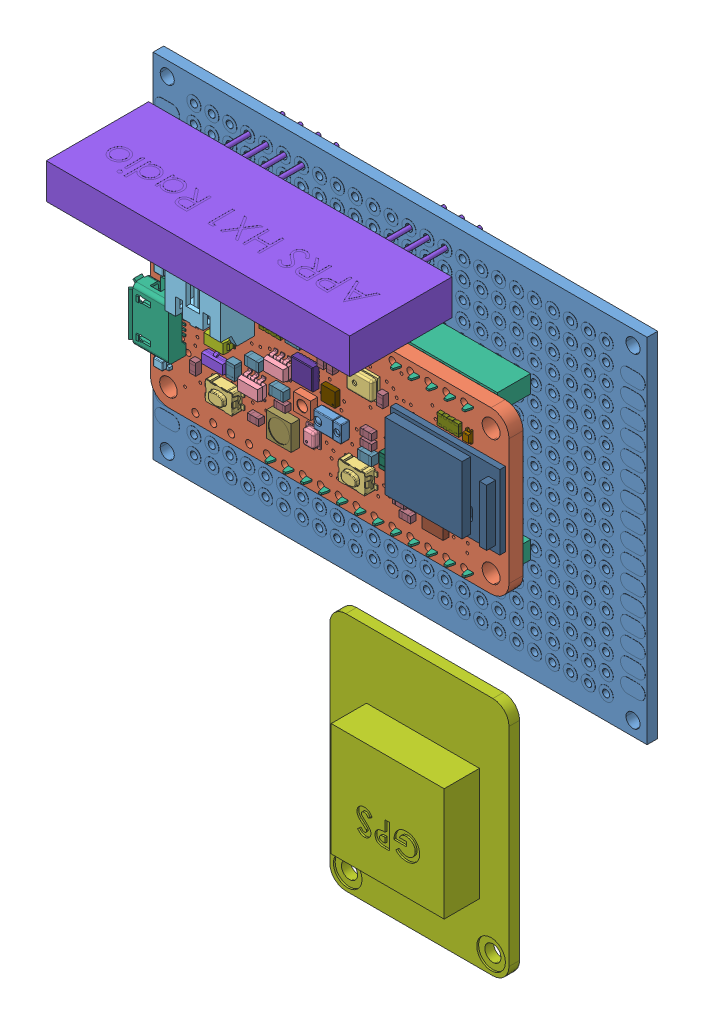
SolidWorks assembly protoboard_assembly, configuration Default. Lengths in mm.
Overall size (70 82.89 26.5).
48 component instances, 26 part files, 16 mates.
Components (placement in the parent):
- protoboard-1: protoboard [Default] at (39.9767 30.2093 49.9679) size (70 50 1.55)
- feather_sense-1: feather_sense [Default] at (11.5967 19.6493 56.4679) size (51.35 22.86 6.79)
  - feather_sense.step-1: feather_sense.step [Default] at origin size (51.35 22.86 6.79)
    - PCB Component.step-1: PCB Component.step [Default] at origin size (51.35 22.86 6.79)
      - Board.step-1: Board.step [Default] at origin size (50.8 22.86 1.99)
      - KMR2.step-1: KMR2.step [Default] at (11.1 6.223 1.99) size (4.6 2.8 1.94)
      - KMR2.step-2: KMR2.step [Default] at (29.934 5.855 1.99) size (4.6 2.8 1.94)
      - AP2112(3.3V).step-1: AP2112(3.3V).step [Default] at (15.138 9.144 1.99) x (-1 0 0) z (0 0 1) size (3 3 1.4)
      - AP2112(3.3V).step-2: AP2112(3.3V).step [Default] at (18.783 13.386 1.99) x (-1 0 0) z (0 0 1) size (3 3 1.4)
      - RED.step-1: RED.step [Default] at (2.083 5.639 1.99) x (0 -1 0) z (0 0 1) size (1.25 2.02 1.1)
      - RED.step-2: RED.step [Default] at (2.222 17.272 1.99) x (0 1 0) z (0 0 1) size (1.25 2.02 1.1)
      - 4u20329.step-1: 4u20329.step [Default] at (4.445 11.43 1.99) x (0 -1 0) z (0 0 1) size (8.8 5.6 3)
      - MBR054.step-1: MBR054.step [Default] at (10.262 12.395 1.99) x (-1 0 0) z (0 0 1) size (3.6 1.4 1.35)
      - DMG2305.step-1: DMG2305.step [Default] at (9.817 9.55 1.99) size (3.04 2.64 1.12)
      - BLUE.step-1: BLUE.step [Default] at (45.339 18.034 1.99) x (-1 0 0) z (0 0 1) size (0.79 1.6 0.71)
      - MDBT50.step-1: MDBT50.step [Default] at (42.545 11.43 1.99) x (0 -1 0) z (0 0 1) size (10.5 15.5 2.05)
      - GD25Q16.step-1: GD25Q16.step [Default] at (40.767 4.953 1.99) x (-1 0 0) z (0 0 1) size (3 2 0.8)
      - WS2812B3535.step-1: WS2812B3535.step [Default] at (19.387 6.145 1.99) x (-1 0 0) z (0 0 1) size (3.5 3.5 1.2)
      - 2.2K.step-1: 2.2K.step [Default] at (19.075 8.788 1.99) size (1.6 0.9 0.8)
      - 2.2K.step-2: 2.2K.step [Default] at (31.306 10.198 1.99) size (1.6 0.9 0.8)
      - 2.2K.step-3: 2.2K.step [Default] at (6.756 7.379 1.99) x (0 1 0) z (0 0 1) size (1.6 0.9 0.8)
      - 2.2K.step-4: 2.2K.step [Default] at (15.316 5.309 1.99) size (1.6 0.9 0.8)
      - 2.2K.step-5: 2.2K.step [Default] at (35.878 5.398 1.99) size (1.6 0.9 0.8)
      - 2.2K.step-6: 2.2K.step [Default] at (36.83 4.128 1.99) size (1.6 0.9 0.8)
      - 2.2K.step-7: 2.2K.step [Default] at (33.274 16.637 1.99) x (0 1 0) z (0 0 1) size (1.6 0.9 0.8)
      - 2.2K.step-8: 2.2K.step [Default] at (26.162 17.208 1.99) x (0 -1 0) z (0 0 1) size (1.6 0.9 0.8)
      - 2.2K.step-9: 2.2K.step [Default] at (31.306 11.494 1.99) size (1.6 0.9 0.8)
      - 2.2K.step-10: 2.2K.step [Default] at (24.828 17.208 1.99) x (0 -1 0) z (0 0 1) size (1.6 0.9 0.8)
      - 2.2K.step-11: 2.2K.step [Default] at (5.715 19.685 1.99) x (0 -1 0) z (0 0 1) size (1.6 0.9 0.8)
      - 10uF.step-1: 10uF.step [Default] at (18.796 10.376 1.99) size (2 1.25 1)
      - 10uF.step-2: 10uF.step [Default] at (21.082 17.907 1.99) x (-1 0 0) z (0 0 1) size (2 1.25 1)
      - 10uF.step-3: 10uF.step [Default] at (12.294 9.855 1.99) x (0 1 0) z (0 0 1) size (2 1.25 1)
      - 10uF.step-4: 10uF.step [Default] at (31.306 8.712 1.99) size (2 1.25 1)
      - 10uF.step-5: 10uF.step [Default] at (15.316 12.256 1.99) x (-1 0 0) z (0 0 1) size (2 1.25 1)
      - DNP.step-1: DNP.step [Default] at (33.82 9.373 1.99) x (0 -1 0) z (0 0 1) size (2 1.25 0.85)
      - 4.7K.step-1: 4.7K.step [Default] at (17.374 17.501 1.99) x (-1 0 0) z (0 0 1) size (3.05 1.6 0.5)
      - 4.7K.step-2: 4.7K.step [Default] at (42.608 18.224 1.99) x (-1 0 0) z (0 0 1) size (3.05 1.6 0.5)
      - LSM6DS33.step-1: LSM6DS33.step [Default] at (22.416 14.542 1.99) x (0 1 0) z (0 0 1) size (3 3 1)
      - LIS3MDL.step-1: LIS3MDL.step [Default] at (25.844 13.398 1.99) x (-1 0 0) z (0 0 1) size (2 2 0.7)
      - APDS-9960.step-1: APDS-9960.step [Default] at (26.352 10.224 1.99) x (0 1 0) z (0 0 1) size (2.36 3.94 1.36)
      - SHT30.step-1: SHT30.step [Default] at (22.479 10.668 1.99) size (2.4 2.4 1)
      - MIC_PDM.step-1: MIC_PDM.step [Default] at (30.544 17.272 1.99) x (0 1 0) z (0 0 1) size (3 4 1.06)
      - BMP280.step-1: BMP280.step [Default] at (23.241 6.985 1.99) x (-1 0 0) z (0 0 1) size (2 2.5 0.97)
      - CON_JST_PH_2PIN_MTPH2.step-1: CON_JST_PH_2PIN_MTPH2.step [Default] at (10.795 19.304 1.99) size (7.9 8.6 4.8)
- 12pin-header-1: 12pin-header [Default] at (42.9767 41.2593 56.4679) x (1 0 0) z (0 1 0) size (30.98 8 2.5)
- 12pin-header-2: 12pin-header [Default] at (42.9767 20.8993 56.4679) x (1 0 0) z (0 1 0) size (30.98 8 2.5)
- ultimate_gps-1: ultimate_gps [Default] at (49.6967 -10.0687 56.9579) x (0 -1 0) z (-1 0 0) size (34.04 6.5 25.4)
- hx1_radio-1: hx1_radio [Default] at (32.8267 50.7993 65.7079) x (-1 0 0) z (0 0 -1) size (43 5 26.5)
Mates (geometry in assembly coordinates):
- Coincident1: coincident anti-aligned: plane of feather_sense-1/feather_sense.step-1/PCB Component.step-1/Board.step-1 through (36.9967 31.0793 56.4679) normal (0 0 -1); plane of 12pin-header-1 through (27.4867 42.5093 56.4679) normal (0 0 1)
- Coincident2: coincident aligned: plane of feather_sense-1/feather_sense.step-1/PCB Component.step-1/Board.step-1 through (59.8567 42.5093 56.4679) normal (0 1 0); plane of 12pin-header-1 through (27.4867 42.5093 51.4679) normal (0 1 0)
- Tangent2: tangent: circle of feather_sense-1/feather_sense.step-1/PCB Component.step-1/Board.step-1; plane of 12pin-header-1 through (56.5467 41.2593 56.4679) normal (-1 0 0)
- Coincident6: coincident anti-aligned: plane of feather_sense-1/feather_sense.step-1/PCB Component.step-1/Board.step-1 through (36.9967 31.0793 56.4679) normal (0 0 -1); plane of 12pin-header-2 through (27.4867 22.1493 56.4679) normal (0 0 1)
- Coincident7: coincident aligned: plane of feather_sense-1/feather_sense.step-1/PCB Component.step-1/Board.step-1 through (14.1367 19.6493 56.4679) normal (0 -1 0); plane of 12pin-header-2 through (27.4867 19.6493 56.4679) normal (0 -1 0)
- Tangent3: tangent: circle of feather_sense-1/feather_sense.step-1/PCB Component.step-1/Board.step-1; plane of 12pin-header-2 through (56.5467 20.8993 56.4679) normal (-1 0 0)
- Coincident10: coincident anti-aligned: plane of protoboard-1 through (39.9767 30.2093 51.4679) normal (0 0 1); plane of 12pin-header-1 through (27.4867 40.0093 51.4679) normal (0 0 -1)
- Parallel2: parallel aligned: plane of protoboard-1 through (4.9767 55.2093 49.9679) normal (0 1 0); plane of 12pin-header-1 through (27.4867 42.5093 51.4679) normal (0 1 0)
- Coincident14: coincident aligned: plane of feather_sense-1/feather_sense.step-1/PCB Component.step-1/Board.step-1 through (36.9967 31.0793 58.4579) normal (0 0 1); plane of ultimate_gps-1 through (49.6967 -10.0687 58.4579) normal (0 0 1)
- Distance1: distance = 12.7 mm anti-aligned: plane of ultimate_gps-1 through (36.9967 6.9493 58.4579) normal (0 1 0); plane of feather_sense-1/feather_sense.step-1/PCB Component.step-1/Board.step-1 through (14.1367 19.6493 56.4679) normal (0 -1 0)
- Coincident16: coincident aligned: plane of feather_sense-1/feather_sense.step-1/PCB Component.step-1/Board.step-1 through (62.3967 22.1893 56.4679) normal (1 0 0); plane of ultimate_gps-1 through (62.3967 6.9493 58.4579) normal (1 0 0)
- Distance2: distance = 12.7 mm aligned: plane of protoboard-1 through (4.9767 55.2093 49.9679) normal (0 1 0); plane of 12pin-header-1 through (27.4867 42.5093 51.4679) normal (0 1 0)
- Distance3: distance = 16.51 mm aligned: plane of 12pin-header-1 through (58.4667 41.2593 56.4679) normal (1 0 0); plane of protoboard-1 through (74.9767 55.2093 49.9679) normal (1 0 0)
- Concentric2: concentric aligned: cylinder of protoboard-1 through (18.3867 51.7993 50.7179) axis (0 0 1) radius 0.5; cylinder of hx1_radio-1 through (18.3867 51.7993 46.4579) axis (0 0 1) radius 0.3
- Concentric3: concentric aligned: cylinder of protoboard-1 through (46.3267 51.7993 50.7179) axis (0 0 1) radius 0.5; cylinder of hx1_radio-1 through (46.3267 51.7993 46.4579) axis (0 0 1) radius 0.3
- Coincident19: coincident anti-aligned: plane of feather_sense-1/feather_sense.step-1/PCB Component.step-1/Board.step-1 through (36.9967 31.0793 58.4579) normal (0 0 1); plane of hx1_radio-1 through (54.3267 55.7993 58.4579) normal (0 0 -1)
